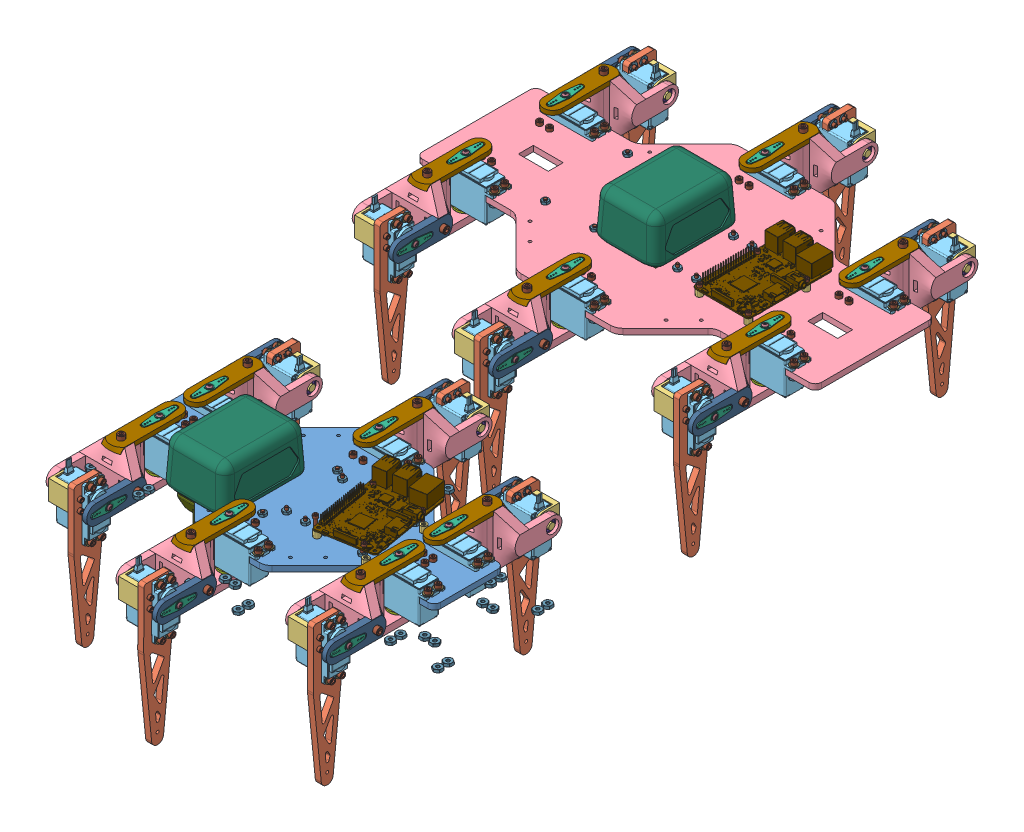
SolidWorks assembly Assem1, configuration Default. Lengths in mm.
Overall size (454.69 181.88 781.08).
774 component instances, 22 part files, 6 mates.
Components (placement in the parent):
- Hexapod_NewBody-1: Hexapod_NewBody [Défaut] at origin size (371.2 181.88 349.28)
  - Body_V2-5: Body_V2 [Default] at (-310 -5.6 15) x (1 0 0) z (0 1 0) size (310 170 5.6)
  - Leg-6: Leg [Default] at (-54.94 -26.67 -0.094) size (70.67 158.62 124.58)
    - Foot_V2_Straight-1: Foot_V2_Straight [Default] at (5.4563 4.661 -91.3712) x (0.005731 -0.001458 0.999983) z (-0.999984 0 0.005731) size (28 145.4 6)
    - bearing_mount_foot-1: bearing_mount_foot [Default] at (5.5782 16.6093 -99.7646) x (-0.005731 0.001458 -0.999983) z (0.999984 0 -0.005731) size (25 20 29.5)
    - Joint-1: Joint [Défaut] at (36.1468 26.4662 -54.5086) x (-0.005731 0 -0.999984) z (0 1 0) size (96.52 53.26 53.26)
    - hs-422-2: hs-422 [Défaut] at (5.505 6.6398 -77.4623) x (-0.005731 0.001458 -0.999983) z (0.000008 0.999999 0.001458) size (19.81 42.09 58.23)
    - hs-422-3: hs-422 [Défaut] at (19.939 20.701 -19.812) x (0 0 1) z (-1 0 0) size (19.81 42.09 58.23)
    - hs-422_horn_straight-1: hs-422_horn_straight [Default] at (-16.4246 16.9412 -87.2278) x (0.005731 0 0.999984) z (0 1 0) size (33.93 4.93 8.79)
    - hs-422_horn_straight-2: hs-422_horn_straight [Default] at (9.652 42.5743 -9.906) x (-0.005731 0 -0.999984) z (-0.999984 0 0.005731) size (33.93 4.93 8.79)
    - Bearing_mount_leg-1: Bearing_mount_leg [Default] at (9.652 21 2.594) x (0 0 1) z (0 -1 0) size (35 20 30)
    - Bearing-1: Bearing [Default] at (9.652 -6.7498 -9.906) x (0.84763 0 0.530588) z (-0.530588 0 0.84763) size (13.87 4.75 13.87)
    - Bearing-2: Bearing [Default] at (32.8986 16.9412 -87.5105) x (0.003061 -0.845349 0.534206) z (-0.004844 -0.534214 -0.845335) size (13.87 4.75 13.87)
    - Joint_attachment_leg-1: Joint_attachment_leg [Défaut] at (36.1468 26.4662 -54.5086) x (-0.005731 0 -0.999984) z (0 1 0) size (74.32 19.07 4.32)
    - Joint_attachment_foot-1: Joint_attachment_foot [Défaut] at (36.1468 26.4662 -54.5086) x (-0.005731 0 -0.999984) z (0 1 0) size (64.08 6.7 19.07)
    - socket_1_2_6-32_with_washer-1: socket_1_2_6-32_with_washer [Défaut] at (43.8172 -14.6702 -93.6435) x (0.999984 0 -0.005731) z (0.004959 -0.501262 0.865281) size (16.21 7.92 7.92)
      - socket head cap screw_ai-1: socket head cap screw_ai [HX-SHCS 0.138-32x0.5x0.5-N] at (-51.206 -1.62 2.0257) size (16.21 5.74 5.74)
      - flat washer type b narrow_ai-1: flat washer type b narrow_ai [Narrow FW 0.138] at (-46.888 -1.62 2.0257) size (0.81 7.92 7.92)
    - socket_1_2_6-32_with_washer-2: socket_1_2_6-32_with_washer [Défaut] at (43.8716 -19.1255 -84.1659) x (0.999984 0 -0.005731) z (0.000008 0.999999 0.001458) size (16.21 7.92 7.92)
      - socket head cap screw_ai-1: socket head cap screw_ai [HX-SHCS 0.138-32x0.5x0.5-N] at (-51.206 -1.62 2.0257) size (16.21 5.74 5.74)
      - flat washer type b narrow_ai-1: flat washer type b narrow_ai [Narrow FW 0.138] at (-46.888 -1.62 2.0257) size (0.81 7.92 7.92)
    - socket_1_2_6-32_with_washer-3: socket_1_2_6-32_with_washer [Défaut] at (43.8284 27.9935 -91.6928) x (0.999984 0 -0.005731) z (-0.004959 0.501262 -0.865281) size (16.21 7.92 7.92)
      - socket head cap screw_ai-1: socket head cap screw_ai [HX-SHCS 0.138-32x0.5x0.5-N] at (-51.206 -1.62 2.0257) size (16.21 5.74 5.74)
      - flat washer type b narrow_ai-1: flat washer type b narrow_ai [Narrow FW 0.138] at (-46.888 -1.62 2.0257) size (0.81 7.92 7.92)
    - socket_1_2_6-32_with_washer-4: socket_1_2_6-32_with_washer [Défaut] at (43.8866 27.9806 -81.533) x (0.999984 0 -0.005731) z (-0.004959 0.501262 -0.865281) size (16.21 7.92 7.92)
      - socket head cap screw_ai-1: socket head cap screw_ai [HX-SHCS 0.138-32x0.5x0.5-N] at (-51.206 -1.62 2.0257) size (16.21 5.74 5.74)
      - flat washer type b narrow_ai-1: flat washer type b narrow_ai [Narrow FW 0.138] at (-46.888 -1.62 2.0257) size (0.81 7.92 7.92)
    - socket button head cap screw_ai-2: socket button head cap screw_ai [SBHCSCREW 0.112-40x0.25-HX-N] at (-19.4218 16.9412 -87.2107) x (0.999984 0 -0.005731) z (-0.002865 0.866025 -0.499992) size (7.85 5.41 5.41)
    - socket button head cap screw_ai-3: socket button head cap screw_ai [SBHCSCREW 0.112-40x0.25-HX-N] at (9.652 45.5715 -9.906) x (0 -1 0) z (0.868877 0 0.495029) size (7.85 5.41 5.41)
    - machine screw nut hex_ai-7: machine screw nut hex_ai [MSHXNUT 0.138-32-D-N] at (5.4499 -17.0874 -92.4829) x (-0.004959 0.501262 -0.865281) z (0.999984 0 -0.005731) size (7.92 9.15 2.9)
    - machine screw nut hex_ai-8: machine screw nut hex_ai [MSHXNUT 0.138-32-D-N] at (5.5081 -17.1022 -82.3231) x (-0.004959 0.501262 -0.865281) z (-0.999984 0 0.005731) size (7.92 9.15 2.9)
    - machine screw nut hex_ai-9: machine screw nut hex_ai [MSHXNUT 0.138-32-D-N] at (5.4503 30.4106 -92.4136) x (0.000008 0.999999 0.001458) z (0.999984 0 -0.005731) size (7.92 9.15 2.9)
    - machine screw nut hex_ai-10: machine screw nut hex_ai [MSHXNUT 0.138-32-D-N] at (5.5085 30.3978 -82.2538) x (0.000008 0.999999 0.001458) z (0.999984 0 -0.005731) size (7.92 9.15 2.9)
    - socket head cap screw_ai-1: socket head cap screw_ai [HX-SHCS 0.164-32x0.5x0.5-N] at (9.4314 47.8568 -48.4033) x (0 -1 0) z (0.005731 0 0.999984) size (16.87 6.86 6.86)
    - socket head cap screw_ai-2: socket head cap screw_ai [HX-SHCS 0.164-32x0.5x0.5-N] at (-21.5482 16.9412 -59.4711) x (0.999984 0 -0.005731) z (0.005731 0 0.999984) size (16.87 6.86 6.86)
    - machine screw nut hex_ai-11: machine screw nut hex_ai [MSHXNUT 0.164-32-D-N] at (9.4314 33.127 -48.4033) x (0.868877 0 0.495029) z (0 1 0) size (8.74 10.09 3.3)
    - machine screw nut hex_ai-12: machine screw nut hex_ai [MSHXNUT 0.164-32-D-N] at (-6.8186 16.9412 -59.5556) x (0.005731 0 0.999984) z (-0.999984 0 0.005731) size (8.74 10.09 3.3)
    - socket head cap screw_ai-3: socket head cap screw_ai [HX-SHCS 0.112-40x0.5x0.5-N] at (-3.4365 11.6733 -99.7202) x (0.999984 0 -0.005731) z (0.005731 -0.001458 0.999983) size (15.54 4.65 4.65)
    - socket head cap screw_ai-4: socket head cap screw_ai [HX-SHCS 0.112-40x0.5x0.5-N] at (-3.4364 21.6733 -99.7056) x (0.999984 0 -0.005731) z (-0.005731 0.001458 -0.999983) size (15.54 4.65 4.65)
    - socket_1_2_6-32_with_washer-5: socket_1_2_6-32_with_washer [Défaut] at (-3.4199 -17.7034 -7.3903) x (0 -1 0) z (0.5 0 0.866025) size (16.21 7.92 7.92)
      - socket head cap screw_ai-1: socket head cap screw_ai [HX-SHCS 0.138-32x0.5x0.5-N] at (-51.206 -1.62 2.0257) size (16.21 5.74 5.74)
      - flat washer type b narrow_ai-1: flat washer type b narrow_ai [Narrow FW 0.138] at (-46.888 -1.62 2.0257) size (0.81 7.92 7.92)
    - socket_1_2_6-32_with_washer-6: socket_1_2_6-32_with_washer [Défaut] at (44.0781 -17.7034 -17.5503) x (0 -1 0) z (0.5 0 0.866025) size (16.21 7.92 7.92)
      - socket head cap screw_ai-1: socket head cap screw_ai [HX-SHCS 0.138-32x0.5x0.5-N] at (-51.206 -1.62 2.0257) size (16.21 5.74 5.74)
      - flat washer type b narrow_ai-1: flat washer type b narrow_ai [Narrow FW 0.138] at (-46.888 -1.62 2.0257) size (0.81 7.92 7.92)
    - socket_1_2_6-32_with_washer-7: socket_1_2_6-32_with_washer [Défaut] at (-3.4199 -17.7034 -17.5503) x (0 -1 0) z (0.5 0 0.866025) size (16.21 7.92 7.92)
      - socket head cap screw_ai-1: socket head cap screw_ai [HX-SHCS 0.138-32x0.5x0.5-N] at (-51.206 -1.62 2.0257) size (16.21 5.74 5.74)
      - flat washer type b narrow_ai-1: flat washer type b narrow_ai [Narrow FW 0.138] at (-46.888 -1.62 2.0257) size (0.81 7.92 7.92)
    - socket_1_2_6-32_with_washer-8: socket_1_2_6-32_with_washer [Défaut] at (44.0781 -17.7034 -7.3903) x (0 -1 0) z (0.5 0 0.866025) size (16.21 7.92 7.92)
      - socket head cap screw_ai-1: socket head cap screw_ai [HX-SHCS 0.138-32x0.5x0.5-N] at (-51.206 -1.62 2.0257) size (16.21 5.74 5.74)
      - flat washer type b narrow_ai-1: flat washer type b narrow_ai [Narrow FW 0.138] at (-46.888 -1.62 2.0257) size (0.81 7.92 7.92)
  - Leg-7: Leg [Default] at (-294.94 -26.67 -0.094) size (70.67 158.62 124.58)
    - Foot_V2_Straight-1: Foot_V2_Straight [Default] at (5.4563 4.661 -91.3712) x (0.005731 -0.001458 0.999983) z (-0.999984 0 0.005731) size (28 145.4 6)
    - bearing_mount_foot-1: bearing_mount_foot [Default] at (5.5782 16.6093 -99.7646) x (-0.005731 0.001458 -0.999983) z (0.999984 0 -0.005731) size (25 20 29.5)
    - Joint-1: Joint [Défaut] at (36.1468 26.4662 -54.5086) x (-0.005731 0 -0.999984) z (0 1 0) size (96.52 53.26 53.26)
    - hs-422-2: hs-422 [Défaut] at (5.505 6.6398 -77.4623) x (-0.005731 0.001458 -0.999983) z (0.000008 0.999999 0.001458) size (19.81 42.09 58.23)
    - hs-422-3: hs-422 [Défaut] at (19.939 20.701 -19.812) x (0 0 1) z (-1 0 0) size (19.81 42.09 58.23)
    - hs-422_horn_straight-1: hs-422_horn_straight [Default] at (-16.4246 16.9412 -87.2278) x (0.005731 0 0.999984) z (0 1 0) size (33.93 4.93 8.79)
    - hs-422_horn_straight-2: hs-422_horn_straight [Default] at (9.652 42.5743 -9.906) x (-0.005731 0 -0.999984) z (-0.999984 0 0.005731) size (33.93 4.93 8.79)
    - Bearing_mount_leg-1: Bearing_mount_leg [Default] at (9.652 21 2.594) x (0 0 1) z (0 -1 0) size (35 20 30)
    - Bearing-1: Bearing [Default] at (9.652 -6.7498 -9.906) x (0.84763 0 0.530588) z (-0.530588 0 0.84763) size (13.87 4.75 13.87)
    - Bearing-2: Bearing [Default] at (32.8986 16.9412 -87.5105) x (0.003061 -0.845349 0.534206) z (-0.004844 -0.534214 -0.845335) size (13.87 4.75 13.87)
    - Joint_attachment_leg-1: Joint_attachment_leg [Défaut] at (36.1468 26.4662 -54.5086) x (-0.005731 0 -0.999984) z (0 1 0) size (74.32 19.07 4.32)
    - Joint_attachment_foot-1: Joint_attachment_foot [Défaut] at (36.1468 26.4662 -54.5086) x (-0.005731 0 -0.999984) z (0 1 0) size (64.08 6.7 19.07)
    - socket_1_2_6-32_with_washer-1: socket_1_2_6-32_with_washer [Défaut] at (43.8172 -14.6702 -93.6435) x (0.999984 0 -0.005731) z (0.004959 -0.501262 0.865281) size (16.21 7.92 7.92)
      - socket head cap screw_ai-1: socket head cap screw_ai [HX-SHCS 0.138-32x0.5x0.5-N] at (-51.206 -1.62 2.0257) size (16.21 5.74 5.74)
      - flat washer type b narrow_ai-1: flat washer type b narrow_ai [Narrow FW 0.138] at (-46.888 -1.62 2.0257) size (0.81 7.92 7.92)
    - socket_1_2_6-32_with_washer-2: socket_1_2_6-32_with_washer [Défaut] at (43.8716 -19.1255 -84.1659) x (0.999984 0 -0.005731) z (0.000008 0.999999 0.001458) size (16.21 7.92 7.92)
      - socket head cap screw_ai-1: socket head cap screw_ai [HX-SHCS 0.138-32x0.5x0.5-N] at (-51.206 -1.62 2.0257) size (16.21 5.74 5.74)
      - flat washer type b narrow_ai-1: flat washer type b narrow_ai [Narrow FW 0.138] at (-46.888 -1.62 2.0257) size (0.81 7.92 7.92)
    - socket_1_2_6-32_with_washer-3: socket_1_2_6-32_with_washer [Défaut] at (43.8284 27.9935 -91.6928) x (0.999984 0 -0.005731) z (-0.004959 0.501262 -0.865281) size (16.21 7.92 7.92)
      - socket head cap screw_ai-1: socket head cap screw_ai [HX-SHCS 0.138-32x0.5x0.5-N] at (-51.206 -1.62 2.0257) size (16.21 5.74 5.74)
      - flat washer type b narrow_ai-1: flat washer type b narrow_ai [Narrow FW 0.138] at (-46.888 -1.62 2.0257) size (0.81 7.92 7.92)
    - socket_1_2_6-32_with_washer-4: socket_1_2_6-32_with_washer [Défaut] at (43.8866 27.9806 -81.533) x (0.999984 0 -0.005731) z (-0.004959 0.501262 -0.865281) size (16.21 7.92 7.92)
      - socket head cap screw_ai-1: socket head cap screw_ai [HX-SHCS 0.138-32x0.5x0.5-N] at (-51.206 -1.62 2.0257) size (16.21 5.74 5.74)
      - flat washer type b narrow_ai-1: flat washer type b narrow_ai [Narrow FW 0.138] at (-46.888 -1.62 2.0257) size (0.81 7.92 7.92)
    - socket button head cap screw_ai-2: socket button head cap screw_ai [SBHCSCREW 0.112-40x0.25-HX-N] at (-19.4218 16.9412 -87.2107) x (0.999984 0 -0.005731) z (-0.002865 0.866025 -0.499992) size (7.85 5.41 5.41)
    - socket button head cap screw_ai-3: socket button head cap screw_ai [SBHCSCREW 0.112-40x0.25-HX-N] at (9.652 45.5715 -9.906) x (0 -1 0) z (0.868877 0 0.495029) size (7.85 5.41 5.41)
    - machine screw nut hex_ai-7: machine screw nut hex_ai [MSHXNUT 0.138-32-D-N] at (5.4499 -17.0874 -92.4829) x (-0.004959 0.501262 -0.865281) z (0.999984 0 -0.005731) size (7.92 9.15 2.9)
    - machine screw nut hex_ai-8: machine screw nut hex_ai [MSHXNUT 0.138-32-D-N] at (5.5081 -17.1022 -82.3231) x (-0.004959 0.501262 -0.865281) z (-0.999984 0 0.005731) size (7.92 9.15 2.9)
    - machine screw nut hex_ai-9: machine screw nut hex_ai [MSHXNUT 0.138-32-D-N] at (5.4503 30.4106 -92.4136) x (0.000008 0.999999 0.001458) z (0.999984 0 -0.005731) size (7.92 9.15 2.9)
    - machine screw nut hex_ai-10: machine screw nut hex_ai [MSHXNUT 0.138-32-D-N] at (5.5085 30.3978 -82.2538) x (0.000008 0.999999 0.001458) z (0.999984 0 -0.005731) size (7.92 9.15 2.9)
    - socket head cap screw_ai-1: socket head cap screw_ai [HX-SHCS 0.164-32x0.5x0.5-N] at (9.4314 47.8568 -48.4033) x (0 -1 0) z (0.005731 0 0.999984) size (16.87 6.86 6.86)
    - socket head cap screw_ai-2: socket head cap screw_ai [HX-SHCS 0.164-32x0.5x0.5-N] at (-21.5482 16.9412 -59.4711) x (0.999984 0 -0.005731) z (0.005731 0 0.999984) size (16.87 6.86 6.86)
    - machine screw nut hex_ai-11: machine screw nut hex_ai [MSHXNUT 0.164-32-D-N] at (9.4314 33.127 -48.4033) x (0.868877 0 0.495029) z (0 1 0) size (8.74 10.09 3.3)
    - machine screw nut hex_ai-12: machine screw nut hex_ai [MSHXNUT 0.164-32-D-N] at (-6.8186 16.9412 -59.5556) x (0.005731 0 0.999984) z (-0.999984 0 0.005731) size (8.74 10.09 3.3)
    - socket head cap screw_ai-3: socket head cap screw_ai [HX-SHCS 0.112-40x0.5x0.5-N] at (-3.4365 11.6733 -99.7202) x (0.999984 0 -0.005731) z (0.005731 -0.001458 0.999983) size (15.54 4.65 4.65)
    - socket head cap screw_ai-4: socket head cap screw_ai [HX-SHCS 0.112-40x0.5x0.5-N] at (-3.4364 21.6733 -99.7056) x (0.999984 0 -0.005731) z (-0.005731 0.001458 -0.999983) size (15.54 4.65 4.65)
    - socket_1_2_6-32_with_washer-5: socket_1_2_6-32_with_washer [Défaut] at (-3.4199 -17.7034 -7.3903) x (0 -1 0) z (0.5 0 0.866025) size (16.21 7.92 7.92)
      - socket head cap screw_ai-1: socket head cap screw_ai [HX-SHCS 0.138-32x0.5x0.5-N] at (-51.206 -1.62 2.0257) size (16.21 5.74 5.74)
      - flat washer type b narrow_ai-1: flat washer type b narrow_ai [Narrow FW 0.138] at (-46.888 -1.62 2.0257) size (0.81 7.92 7.92)
    - socket_1_2_6-32_with_washer-6: socket_1_2_6-32_with_washer [Défaut] at (44.0781 -17.7034 -17.5503) x (0 -1 0) z (0.5 0 0.866025) size (16.21 7.92 7.92)
      - socket head cap screw_ai-1: socket head cap screw_ai [HX-SHCS 0.138-32x0.5x0.5-N] at (-51.206 -1.62 2.0257) size (16.21 5.74 5.74)
      - flat washer type b narrow_ai-1: flat washer type b narrow_ai [Narrow FW 0.138] at (-46.888 -1.62 2.0257) size (0.81 7.92 7.92)
    - socket_1_2_6-32_with_washer-7: socket_1_2_6-32_with_washer [Défaut] at (-3.4199 -17.7034 -17.5503) x (0 -1 0) z (0.5 0 0.866025) size (16.21 7.92 7.92)
      - socket head cap screw_ai-1: socket head cap screw_ai [HX-SHCS 0.138-32x0.5x0.5-N] at (-51.206 -1.62 2.0257) size (16.21 5.74 5.74)
      - flat washer type b narrow_ai-1: flat washer type b narrow_ai [Narrow FW 0.138] at (-46.888 -1.62 2.0257) size (0.81 7.92 7.92)
    - socket_1_2_6-32_with_washer-8: socket_1_2_6-32_with_washer [Défaut] at (44.0781 -17.7034 -7.3903) x (0 -1 0) z (0.5 0 0.866025) size (16.21 7.92 7.92)
      - socket head cap screw_ai-1: socket head cap screw_ai [HX-SHCS 0.138-32x0.5x0.5-N] at (-51.206 -1.62 2.0257) size (16.21 5.74 5.74)
      - flat washer type b narrow_ai-1: flat washer type b narrow_ai [Narrow FW 0.138] at (-46.888 -1.62 2.0257) size (0.81 7.92 7.92)
  - Leg-8: Leg [Default] at (-174.94 -26.67 -50.094) size (70.67 158.62 124.58)
    - Foot_V2_Straight-1: Foot_V2_Straight [Default] at (5.4563 4.661 -91.3712) x (0.005731 -0.001458 0.999983) z (-0.999984 0 0.005731) size (28 145.4 6)
    - bearing_mount_foot-1: bearing_mount_foot [Default] at (5.5782 16.6093 -99.7646) x (-0.005731 0.001458 -0.999983) z (0.999984 0 -0.005731) size (25 20 29.5)
    - Joint-1: Joint [Défaut] at (36.1468 26.4662 -54.5086) x (-0.005731 0 -0.999984) z (0 1 0) size (96.52 53.26 53.26)
    - hs-422-2: hs-422 [Défaut] at (5.505 6.6398 -77.4623) x (-0.005731 0.001458 -0.999983) z (0.000008 0.999999 0.001458) size (19.81 42.09 58.23)
    - hs-422-3: hs-422 [Défaut] at (19.939 20.701 -19.812) x (0 0 1) z (-1 0 0) size (19.81 42.09 58.23)
    - hs-422_horn_straight-1: hs-422_horn_straight [Default] at (-16.4246 16.9412 -87.2278) x (0.005731 0 0.999984) z (0 1 0) size (33.93 4.93 8.79)
    - hs-422_horn_straight-2: hs-422_horn_straight [Default] at (9.652 42.5743 -9.906) x (-0.005731 0 -0.999984) z (-0.999984 0 0.005731) size (33.93 4.93 8.79)
    - Bearing_mount_leg-1: Bearing_mount_leg [Default] at (9.652 21 2.594) x (0 0 1) z (0 -1 0) size (35 20 30)
    - Bearing-1: Bearing [Default] at (9.652 -6.7498 -9.906) x (0.84763 0 0.530588) z (-0.530588 0 0.84763) size (13.87 4.75 13.87)
    - Bearing-2: Bearing [Default] at (32.8986 16.9412 -87.5105) x (0.003061 -0.845349 0.534206) z (-0.004844 -0.534214 -0.845335) size (13.87 4.75 13.87)
    - Joint_attachment_leg-1: Joint_attachment_leg [Défaut] at (36.1468 26.4662 -54.5086) x (-0.005731 0 -0.999984) z (0 1 0) size (74.32 19.07 4.32)
    - Joint_attachment_foot-1: Joint_attachment_foot [Défaut] at (36.1468 26.4662 -54.5086) x (-0.005731 0 -0.999984) z (0 1 0) size (64.08 6.7 19.07)
    - socket_1_2_6-32_with_washer-1: socket_1_2_6-32_with_washer [Défaut] at (43.8172 -14.6702 -93.6435) x (0.999984 0 -0.005731) z (0.004959 -0.501262 0.865281) size (16.21 7.92 7.92)
      - socket head cap screw_ai-1: socket head cap screw_ai [HX-SHCS 0.138-32x0.5x0.5-N] at (-51.206 -1.62 2.0257) size (16.21 5.74 5.74)
      - flat washer type b narrow_ai-1: flat washer type b narrow_ai [Narrow FW 0.138] at (-46.888 -1.62 2.0257) size (0.81 7.92 7.92)
    - socket_1_2_6-32_with_washer-2: socket_1_2_6-32_with_washer [Défaut] at (43.8716 -19.1255 -84.1659) x (0.999984 0 -0.005731) z (0.000008 0.999999 0.001458) size (16.21 7.92 7.92)
      - socket head cap screw_ai-1: socket head cap screw_ai [HX-SHCS 0.138-32x0.5x0.5-N] at (-51.206 -1.62 2.0257) size (16.21 5.74 5.74)
      - flat washer type b narrow_ai-1: flat washer type b narrow_ai [Narrow FW 0.138] at (-46.888 -1.62 2.0257) size (0.81 7.92 7.92)
    - socket_1_2_6-32_with_washer-3: socket_1_2_6-32_with_washer [Défaut] at (43.8284 27.9935 -91.6928) x (0.999984 0 -0.005731) z (-0.004959 0.501262 -0.865281) size (16.21 7.92 7.92)
      - socket head cap screw_ai-1: socket head cap screw_ai [HX-SHCS 0.138-32x0.5x0.5-N] at (-51.206 -1.62 2.0257) size (16.21 5.74 5.74)
      - flat washer type b narrow_ai-1: flat washer type b narrow_ai [Narrow FW 0.138] at (-46.888 -1.62 2.0257) size (0.81 7.92 7.92)
    - socket_1_2_6-32_with_washer-4: socket_1_2_6-32_with_washer [Défaut] at (43.8866 27.9806 -81.533) x (0.999984 0 -0.005731) z (-0.004959 0.501262 -0.865281) size (16.21 7.92 7.92)
      - socket head cap screw_ai-1: socket head cap screw_ai [HX-SHCS 0.138-32x0.5x0.5-N] at (-51.206 -1.62 2.0257) size (16.21 5.74 5.74)
      - flat washer type b narrow_ai-1: flat washer type b narrow_ai [Narrow FW 0.138] at (-46.888 -1.62 2.0257) size (0.81 7.92 7.92)
    - socket button head cap screw_ai-2: socket button head cap screw_ai [SBHCSCREW 0.112-40x0.25-HX-N] at (-19.4218 16.9412 -87.2107) x (0.999984 0 -0.005731) z (-0.002865 0.866025 -0.499992) size (7.85 5.41 5.41)
    - socket button head cap screw_ai-3: socket button head cap screw_ai [SBHCSCREW 0.112-40x0.25-HX-N] at (9.652 45.5715 -9.906) x (0 -1 0) z (0.868877 0 0.495029) size (7.85 5.41 5.41)
    - machine screw nut hex_ai-7: machine screw nut hex_ai [MSHXNUT 0.138-32-D-N] at (5.4499 -17.0874 -92.4829) x (-0.004959 0.501262 -0.865281) z (0.999984 0 -0.005731) size (7.92 9.15 2.9)
    - machine screw nut hex_ai-8: machine screw nut hex_ai [MSHXNUT 0.138-32-D-N] at (5.5081 -17.1022 -82.3231) x (-0.004959 0.501262 -0.865281) z (-0.999984 0 0.005731) size (7.92 9.15 2.9)
    - machine screw nut hex_ai-9: machine screw nut hex_ai [MSHXNUT 0.138-32-D-N] at (5.4503 30.4106 -92.4136) x (0.000008 0.999999 0.001458) z (0.999984 0 -0.005731) size (7.92 9.15 2.9)
    - machine screw nut hex_ai-10: machine screw nut hex_ai [MSHXNUT 0.138-32-D-N] at (5.5085 30.3978 -82.2538) x (0.000008 0.999999 0.001458) z (0.999984 0 -0.005731) size (7.92 9.15 2.9)
    - socket head cap screw_ai-1: socket head cap screw_ai [HX-SHCS 0.164-32x0.5x0.5-N] at (9.4314 47.8568 -48.4033) x (0 -1 0) z (0.005731 0 0.999984) size (16.87 6.86 6.86)
    - socket head cap screw_ai-2: socket head cap screw_ai [HX-SHCS 0.164-32x0.5x0.5-N] at (-21.5482 16.9412 -59.4711) x (0.999984 0 -0.005731) z (0.005731 0 0.999984) size (16.87 6.86 6.86)
    - machine screw nut hex_ai-11: machine screw nut hex_ai [MSHXNUT 0.164-32-D-N] at (9.4314 33.127 -48.4033) x (0.868877 0 0.495029) z (0 1 0) size (8.74 10.09 3.3)
    - machine screw nut hex_ai-12: machine screw nut hex_ai [MSHXNUT 0.164-32-D-N] at (-6.8186 16.9412 -59.5556) x (0.005731 0 0.999984) z (-0.999984 0 0.005731) size (8.74 10.09 3.3)
    - socket head cap screw_ai-3: socket head cap screw_ai [HX-SHCS 0.112-40x0.5x0.5-N] at (-3.4365 11.6733 -99.7202) x (0.999984 0 -0.005731) z (0.005731 -0.001458 0.999983) size (15.54 4.65 4.65)
    - socket head cap screw_ai-4: socket head cap screw_ai [HX-SHCS 0.112-40x0.5x0.5-N] at (-3.4364 21.6733 -99.7056) x (0.999984 0 -0.005731) z (-0.005731 0.001458 -0.999983) size (15.54 4.65 4.65)
    - socket_1_2_6-32_with_washer-5: socket_1_2_6-32_with_washer [Défaut] at (-3.4199 -17.7034 -7.3903) x (0 -1 0) z (0.5 0 0.866025) size (16.21 7.92 7.92)
      - socket head cap screw_ai-1: socket head cap screw_ai [HX-SHCS 0.138-32x0.5x0.5-N] at (-51.206 -1.62 2.0257) size (16.21 5.74 5.74)
      - flat washer type b narrow_ai-1: flat washer type b narrow_ai [Narrow FW 0.138] at (-46.888 -1.62 2.0257) size (0.81 7.92 7.92)
    - socket_1_2_6-32_with_washer-6: socket_1_2_6-32_with_washer [Défaut] at (44.0781 -17.7034 -17.5503) x (0 -1 0) z (0.5 0 0.866025) size (16.21 7.92 7.92)
      - socket head cap screw_ai-1: socket head cap screw_ai [HX-SHCS 0.138-32x0.5x0.5-N] at (-51.206 -1.62 2.0257) size (16.21 5.74 5.74)
      - flat washer type b narrow_ai-1: flat washer type b narrow_ai [Narrow FW 0.138] at (-46.888 -1.62 2.0257) size (0.81 7.92 7.92)
    - socket_1_2_6-32_with_washer-7: socket_1_2_6-32_with_washer [Défaut] at (-3.4199 -17.7034 -17.5503) x (0 -1 0) z (0.5 0 0.866025) size (16.21 7.92 7.92)
      - socket head cap screw_ai-1: socket head cap screw_ai [HX-SHCS 0.138-32x0.5x0.5-N] at (-51.206 -1.62 2.0257) size (16.21 5.74 5.74)
      - flat washer type b narrow_ai-1: flat washer type b narrow_ai [Narrow FW 0.138] at (-46.888 -1.62 2.0257) size (0.81 7.92 7.92)
    - socket_1_2_6-32_with_washer-8: socket_1_2_6-32_with_washer [Défaut] at (44.0781 -17.7034 -7.3903) x (0 -1 0) z (0.5 0 0.866025) size (16.21 7.92 7.92)
      - socket head cap screw_ai-1: socket head cap screw_ai [HX-SHCS 0.138-32x0.5x0.5-N] at (-51.206 -1.62 2.0257) size (16.21 5.74 5.74)
      - flat washer type b narrow_ai-1: flat washer type b narrow_ai [Narrow FW 0.138] at (-46.888 -1.62 2.0257) size (0.81 7.92 7.92)
  - Leg_V2(Mirror)-4: Leg_V2(Mirror) [Default] at (-294.94 -26.67 30.094) x (-1 0 0) z (0 0 -1) size (66.23 158.62 124.7)
    - Foot_V2_Straight-1: Foot_V2_Straight [Default] at (-13.3652 4.661 -91.3946) x (-0.000191 -0.001458 0.999999) z (-1 0 -0.000191) size (28 145.4 6)
    - bearing_mount_foot-1: bearing_mount_foot [Default] at (-13.1936 16.6093 -99.7872) x (0.000191 0.001458 -0.999999) z (1 0 0.000191) size (25 20 29.5)
    - Joint-1: Joint [Défaut] at (17.1065 26.4662 -54.3509) x (0.000191 0 -1) z (0 1 0) size (96.52 53.26 53.26)
    - hs-422-2: hs-422 [Défaut] at (-13.3989 6.6398 -77.4857) x (0.000191 0.001458 -0.999999) z (0 0.999999 0.001458) size (19.81 42.09 58.23)
    - hs-422-3: hs-422 [Défaut] at (-19.939 20.701 0) x (0 0 -1) z (1 0 0) size (19.81 42.09 58.23)
    - hs-422_horn_straight-1: hs-422_horn_straight [Default] at (-35.2703 16.9412 -87.3809) x (-0.000191 0 1) z (0 1 0) size (33.93 4.93 8.79)
    - hs-422_horn_straight-2: hs-422_horn_straight [Default] at (-9.652 42.5743 -9.906) x (0.000191 0 -1) z (-1 0 -0.000191) size (33.93 4.93 8.79)
    - Bearing_mount_leg-1: Bearing_mount_leg [Default] at (-9.652 21 2.594) x (0 0 1) z (0 -1 0) size (35 20 30)
    - Bearing-1: Bearing [Default] at (-9.652 -6.7498 -9.906) x (0.84763 0 0.530588) z (-0.530588 0 0.84763) size (13.87 4.75 13.87)
    - Bearing-2: Bearing [Default] at (14.0538 16.9412 -87.3715) x (-0.000107 0.826531 0.562891) z (-0.000158 -0.562891 0.826531) size (13.87 4.75 13.87)
    - Joint_attachment_leg-1: Joint_attachment_leg [Défaut] at (17.1065 26.4662 -54.3509) x (0.000191 0 -1) z (0 1 0) size (74.32 19.07 4.32)
    - Joint_attachment_foot-1: Joint_attachment_foot [Défaut] at (17.1065 26.4662 -54.3509) x (0.000191 0 -1) z (0 1 0) size (64.08 6.7 19.07)
    - socket_1_2_6-32_with_washer-1: socket_1_2_6-32_with_washer [Défaut] at (25.0085 -14.6702 -93.4398) x (1 0 0.000191) z (-0.000165 -0.501262 0.865296) size (16.21 7.92 7.92)
      - socket head cap screw_ai-1: socket head cap screw_ai [HX-SHCS 0.138-32x0.5x0.5-N] at (-51.206 -1.62 2.0257) size (16.21 5.74 5.74)
      - flat washer type b narrow_ai-1: flat washer type b narrow_ai [Narrow FW 0.138] at (-46.888 -1.62 2.0257) size (0.81 7.92 7.92)
    - socket_1_2_6-32_with_washer-2: socket_1_2_6-32_with_washer [Défaut] at (25.0067 -19.1255 -83.9619) x (1 0 0.000191) z (0 0.999999 0.001458) size (16.21 7.92 7.92)
      - socket head cap screw_ai-1: socket head cap screw_ai [HX-SHCS 0.138-32x0.5x0.5-N] at (-51.206 -1.62 2.0257) size (16.21 5.74 5.74)
      - flat washer type b narrow_ai-1: flat washer type b narrow_ai [Narrow FW 0.138] at (-46.888 -1.62 2.0257) size (0.81 7.92 7.92)
    - socket_1_2_6-32_with_washer-3: socket_1_2_6-32_with_washer [Défaut] at (25.0081 27.9935 -91.489) x (1 0 0.000191) z (0.000165 0.501262 -0.865296) size (16.21 7.92 7.92)
      - socket head cap screw_ai-1: socket head cap screw_ai [HX-SHCS 0.138-32x0.5x0.5-N] at (-51.206 -1.62 2.0257) size (16.21 5.74 5.74)
      - flat washer type b narrow_ai-1: flat washer type b narrow_ai [Narrow FW 0.138] at (-46.888 -1.62 2.0257) size (0.81 7.92 7.92)
    - socket_1_2_6-32_with_washer-4: socket_1_2_6-32_with_washer [Défaut] at (25.0062 27.9806 -81.329) x (1 0 0.000191) z (0.000165 0.501262 -0.865296) size (16.21 7.92 7.92)
      - socket head cap screw_ai-1: socket head cap screw_ai [HX-SHCS 0.138-32x0.5x0.5-N] at (-51.206 -1.62 2.0257) size (16.21 5.74 5.74)
      - flat washer type b narrow_ai-1: flat washer type b narrow_ai [Narrow FW 0.138] at (-46.888 -1.62 2.0257) size (0.81 7.92 7.92)
    - socket button head cap screw_ai-2: socket button head cap screw_ai [SBHCSCREW 0.112-40x0.25-HX-N] at (-38.2675 16.9412 -87.3815) x (1 0 0.000191) z (0.000095 0.866025 -0.5) size (7.85 5.41 5.41)
    - socket button head cap screw_ai-3: socket button head cap screw_ai [SBHCSCREW 0.112-40x0.25-HX-N] at (-9.652 45.5715 -9.906) x (0 -1 0) z (0.86593 0 0.500165) size (7.85 5.41 5.41)
    - machine screw nut hex_ai-7: machine screw nut hex_ai [MSHXNUT 0.138-32-D-N] at (-13.365 -17.0874 -92.5063) x (0.000165 0.501262 -0.865296) z (1 0 0.000191) size (7.92 9.15 2.9)
    - machine screw nut hex_ai-8: machine screw nut hex_ai [MSHXNUT 0.138-32-D-N] at (-13.367 -17.1022 -82.3463) x (0.000165 0.501262 -0.865296) z (-1 0 -0.000191) size (7.92 9.15 2.9)
    - machine screw nut hex_ai-9: machine screw nut hex_ai [MSHXNUT 0.138-32-D-N] at (-13.3651 30.4106 -92.4371) x (0 0.999999 0.001458) z (1 0 0.000191) size (7.92 9.15 2.9)
    - machine screw nut hex_ai-10: machine screw nut hex_ai [MSHXNUT 0.138-32-D-N] at (-13.367 30.3978 -82.2771) x (0 0.999999 0.001458) z (1 0 0.000191) size (7.92 9.15 2.9)
    - socket head cap screw_ai-1: socket head cap screw_ai [HX-SHCS 0.164-32x0.5x0.5-N] at (-9.6447 47.8568 -48.4039) x (0 -1 0) z (-0.000191 0 1) size (16.87 6.86 6.86)
    - socket head cap screw_ai-2: socket head cap screw_ai [HX-SHCS 0.164-32x0.5x0.5-N] at (-40.5581 16.9412 -59.655) x (1 0 0.000191) z (-0.000191 0 1) size (16.87 6.86 6.86)
    - machine screw nut hex_ai-11: machine screw nut hex_ai [MSHXNUT 0.164-32-D-N] at (-9.6447 33.127 -48.4039) x (0.86593 0 0.500165) z (0 1 0) size (8.74 10.09 3.3)
    - machine screw nut hex_ai-12: machine screw nut hex_ai [MSHXNUT 0.164-32-D-N] at (-25.8283 16.9412 -59.6522) x (-0.000191 0 1) z (-1 0 -0.000191) size (8.74 10.09 3.3)
    - socket head cap screw_ai-3: socket head cap screw_ai [HX-SHCS 0.112-40x0.5x0.5-N] at (-22.2084 11.6733 -99.7961) x (1 0 0.000191) z (-0.000191 -0.001458 0.999999) size (15.54 4.65 4.65)
    - socket head cap screw_ai-4: socket head cap screw_ai [HX-SHCS 0.112-40x0.5x0.5-N] at (-22.2084 21.6733 -99.7815) x (1 0 0.000191) z (0.000191 0.001458 -0.999999) size (15.54 4.65 4.65)
    - socket_1_2_6-32_with_washer-5: socket_1_2_6-32_with_washer [Défaut] at (3.4199 -17.7034 -12.4217) x (0 -1 0) z (-0.5 0 -0.866025) size (16.21 7.92 7.92)
      - socket head cap screw_ai-1: socket head cap screw_ai [HX-SHCS 0.138-32x0.5x0.5-N] at (-51.206 -1.62 2.0257) size (16.21 5.74 5.74)
      - flat washer type b narrow_ai-1: flat washer type b narrow_ai [Narrow FW 0.138] at (-46.888 -1.62 2.0257) size (0.81 7.92 7.92)
    - socket_1_2_6-32_with_washer-6: socket_1_2_6-32_with_washer [Défaut] at (-44.0781 -17.7034 -2.2617) x (0 -1 0) z (-0.5 0 -0.866025) size (16.21 7.92 7.92)
      - socket head cap screw_ai-1: socket head cap screw_ai [HX-SHCS 0.138-32x0.5x0.5-N] at (-51.206 -1.62 2.0257) size (16.21 5.74 5.74)
      - flat washer type b narrow_ai-1: flat washer type b narrow_ai [Narrow FW 0.138] at (-46.888 -1.62 2.0257) size (0.81 7.92 7.92)
    - socket_1_2_6-32_with_washer-7: socket_1_2_6-32_with_washer [Défaut] at (3.4199 -17.7034 -2.2617) x (0 -1 0) z (-0.5 0 -0.866025) size (16.21 7.92 7.92)
      - socket head cap screw_ai-1: socket head cap screw_ai [HX-SHCS 0.138-32x0.5x0.5-N] at (-51.206 -1.62 2.0257) size (16.21 5.74 5.74)
      - flat washer type b narrow_ai-1: flat washer type b narrow_ai [Narrow FW 0.138] at (-46.888 -1.62 2.0257) size (0.81 7.92 7.92)
    - socket_1_2_6-32_with_washer-8: socket_1_2_6-32_with_washer [Défaut] at (-44.0781 -17.7034 -12.4217) x (0 -1 0) z (-0.5 0 -0.866025) size (16.21 7.92 7.92)
      - socket head cap screw_ai-1: socket head cap screw_ai [HX-SHCS 0.138-32x0.5x0.5-N] at (-51.206 -1.62 2.0257) size (16.21 5.74 5.74)
      - flat washer type b narrow_ai-1: flat washer type b narrow_ai [Narrow FW 0.138] at (-46.888 -1.62 2.0257) size (0.81 7.92 7.92)
  - Leg_V2(Mirror)-5: Leg_V2(Mirror) [Default] at (-54.94 -26.67 30.094) x (-1 0 0) z (0 0 -1) size (66.23 158.62 124.7)
    - Foot_V2_Straight-1: Foot_V2_Straight [Default] at (-13.3652 4.661 -91.3946) x (-0.000191 -0.001458 0.999999) z (-1 0 -0.000191) size (28 145.4 6)
    - bearing_mount_foot-1: bearing_mount_foot [Default] at (-13.1936 16.6093 -99.7872) x (0.000191 0.001458 -0.999999) z (1 0 0.000191) size (25 20 29.5)
    - Joint-1: Joint [Défaut] at (17.1065 26.4662 -54.3509) x (0.000191 0 -1) z (0 1 0) size (96.52 53.26 53.26)
    - hs-422-2: hs-422 [Défaut] at (-13.3989 6.6398 -77.4857) x (0.000191 0.001458 -0.999999) z (0 0.999999 0.001458) size (19.81 42.09 58.23)
    - hs-422-3: hs-422 [Défaut] at (-19.939 20.701 0) x (0 0 -1) z (1 0 0) size (19.81 42.09 58.23)
    - hs-422_horn_straight-1: hs-422_horn_straight [Default] at (-35.2703 16.9412 -87.3809) x (-0.000191 0 1) z (0 1 0) size (33.93 4.93 8.79)
    - hs-422_horn_straight-2: hs-422_horn_straight [Default] at (-9.652 42.5743 -9.906) x (0.000191 0 -1) z (-1 0 -0.000191) size (33.93 4.93 8.79)
    - Bearing_mount_leg-1: Bearing_mount_leg [Default] at (-9.652 21 2.594) x (0 0 1) z (0 -1 0) size (35 20 30)
    - Bearing-1: Bearing [Default] at (-9.652 -6.7498 -9.906) x (0.84763 0 0.530588) z (-0.530588 0 0.84763) size (13.87 4.75 13.87)
    - Bearing-2: Bearing [Default] at (14.0538 16.9412 -87.3715) x (-0.000107 0.826531 0.562891) z (-0.000158 -0.562891 0.826531) size (13.87 4.75 13.87)
    - Joint_attachment_leg-1: Joint_attachment_leg [Défaut] at (17.1065 26.4662 -54.3509) x (0.000191 0 -1) z (0 1 0) size (74.32 19.07 4.32)
    - Joint_attachment_foot-1: Joint_attachment_foot [Défaut] at (17.1065 26.4662 -54.3509) x (0.000191 0 -1) z (0 1 0) size (64.08 6.7 19.07)
    - socket_1_2_6-32_with_washer-1: socket_1_2_6-32_with_washer [Défaut] at (25.0085 -14.6702 -93.4398) x (1 0 0.000191) z (-0.000165 -0.501262 0.865296) size (16.21 7.92 7.92)
      - socket head cap screw_ai-1: socket head cap screw_ai [HX-SHCS 0.138-32x0.5x0.5-N] at (-51.206 -1.62 2.0257) size (16.21 5.74 5.74)
      - flat washer type b narrow_ai-1: flat washer type b narrow_ai [Narrow FW 0.138] at (-46.888 -1.62 2.0257) size (0.81 7.92 7.92)
    - socket_1_2_6-32_with_washer-2: socket_1_2_6-32_with_washer [Défaut] at (25.0067 -19.1255 -83.9619) x (1 0 0.000191) z (0 0.999999 0.001458) size (16.21 7.92 7.92)
      - socket head cap screw_ai-1: socket head cap screw_ai [HX-SHCS 0.138-32x0.5x0.5-N] at (-51.206 -1.62 2.0257) size (16.21 5.74 5.74)
      - flat washer type b narrow_ai-1: flat washer type b narrow_ai [Narrow FW 0.138] at (-46.888 -1.62 2.0257) size (0.81 7.92 7.92)
    - socket_1_2_6-32_with_washer-3: socket_1_2_6-32_with_washer [Défaut] at (25.0081 27.9935 -91.489) x (1 0 0.000191) z (0.000165 0.501262 -0.865296) size (16.21 7.92 7.92)
      - socket head cap screw_ai-1: socket head cap screw_ai [HX-SHCS 0.138-32x0.5x0.5-N] at (-51.206 -1.62 2.0257) size (16.21 5.74 5.74)
      - flat washer type b narrow_ai-1: flat washer type b narrow_ai [Narrow FW 0.138] at (-46.888 -1.62 2.0257) size (0.81 7.92 7.92)
    - socket_1_2_6-32_with_washer-4: socket_1_2_6-32_with_washer [Défaut] at (25.0062 27.9806 -81.329) x (1 0 0.000191) z (0.000165 0.501262 -0.865296) size (16.21 7.92 7.92)
      - socket head cap screw_ai-1: socket head cap screw_ai [HX-SHCS 0.138-32x0.5x0.5-N] at (-51.206 -1.62 2.0257) size (16.21 5.74 5.74)
      - flat washer type b narrow_ai-1: flat washer type b narrow_ai [Narrow FW 0.138] at (-46.888 -1.62 2.0257) size (0.81 7.92 7.92)
    - socket button head cap screw_ai-2: socket button head cap screw_ai [SBHCSCREW 0.112-40x0.25-HX-N] at (-38.2675 16.9412 -87.3815) x (1 0 0.000191) z (0.000095 0.866025 -0.5) size (7.85 5.41 5.41)
    - socket button head cap screw_ai-3: socket button head cap screw_ai [SBHCSCREW 0.112-40x0.25-HX-N] at (-9.652 45.5715 -9.906) x (0 -1 0) z (0.86593 0 0.500165) size (7.85 5.41 5.41)
    - machine screw nut hex_ai-7: machine screw nut hex_ai [MSHXNUT 0.138-32-D-N] at (-13.365 -17.0874 -92.5063) x (0.000165 0.501262 -0.865296) z (1 0 0.000191) size (7.92 9.15 2.9)
    - machine screw nut hex_ai-8: machine screw nut hex_ai [MSHXNUT 0.138-32-D-N] at (-13.367 -17.1022 -82.3463) x (0.000165 0.501262 -0.865296) z (-1 0 -0.000191) size (7.92 9.15 2.9)
    - machine screw nut hex_ai-9: machine screw nut hex_ai [MSHXNUT 0.138-32-D-N] at (-13.3651 30.4106 -92.4371) x (0 0.999999 0.001458) z (1 0 0.000191) size (7.92 9.15 2.9)
    - machine screw nut hex_ai-10: machine screw nut hex_ai [MSHXNUT 0.138-32-D-N] at (-13.367 30.3978 -82.2771) x (0 0.999999 0.001458) z (1 0 0.000191) size (7.92 9.15 2.9)
    - socket head cap screw_ai-1: socket head cap screw_ai [HX-SHCS 0.164-32x0.5x0.5-N] at (-9.6447 47.8568 -48.4039) x (0 -1 0) z (-0.000191 0 1) size (16.87 6.86 6.86)
    - socket head cap screw_ai-2: socket head cap screw_ai [HX-SHCS 0.164-32x0.5x0.5-N] at (-40.5581 16.9412 -59.655) x (1 0 0.000191) z (-0.000191 0 1) size (16.87 6.86 6.86)
    - machine screw nut hex_ai-11: machine screw nut hex_ai [MSHXNUT 0.164-32-D-N] at (-9.6447 33.127 -48.4039) x (0.86593 0 0.500165) z (0 1 0) size (8.74 10.09 3.3)
    - machine screw nut hex_ai-12: machine screw nut hex_ai [MSHXNUT 0.164-32-D-N] at (-25.8283 16.9412 -59.6522) x (-0.000191 0 1) z (-1 0 -0.000191) size (8.74 10.09 3.3)
    - socket head cap screw_ai-3: socket head cap screw_ai [HX-SHCS 0.112-40x0.5x0.5-N] at (-22.2084 11.6733 -99.7961) x (1 0 0.000191) z (-0.000191 -0.001458 0.999999) size (15.54 4.65 4.65)
    - socket head cap screw_ai-4: socket head cap screw_ai [HX-SHCS 0.112-40x0.5x0.5-N] at (-22.2084 21.6733 -99.7815) x (1 0 0.000191) z (0.000191 0.001458 -0.999999) size (15.54 4.65 4.65)
    - socket_1_2_6-32_with_washer-5: socket_1_2_6-32_with_washer [Défaut] at (3.4199 -17.7034 -12.4217) x (0 -1 0) z (-0.5 0 -0.866025) size (16.21 7.92 7.92)
      - socket head cap screw_ai-1: socket head cap screw_ai [HX-SHCS 0.138-32x0.5x0.5-N] at (-51.206 -1.62 2.0257) size (16.21 5.74 5.74)
      - flat washer type b narrow_ai-1: flat washer type b narrow_ai [Narrow FW 0.138] at (-46.888 -1.62 2.0257) size (0.81 7.92 7.92)
    - socket_1_2_6-32_with_washer-6: socket_1_2_6-32_with_washer [Défaut] at (-44.0781 -17.7034 -2.2617) x (0 -1 0) z (-0.5 0 -0.866025) size (16.21 7.92 7.92)
      - socket head cap screw_ai-1: socket head cap screw_ai [HX-SHCS 0.138-32x0.5x0.5-N] at (-51.206 -1.62 2.0257) size (16.21 5.74 5.74)
      - flat washer type b narrow_ai-1: flat washer type b narrow_ai [Narrow FW 0.138] at (-46.888 -1.62 2.0257) size (0.81 7.92 7.92)
    - socket_1_2_6-32_with_washer-7: socket_1_2_6-32_with_washer [Défaut] at (3.4199 -17.7034 -2.2617) x (0 -1 0) z (-0.5 0 -0.866025) size (16.21 7.92 7.92)
      - socket head cap screw_ai-1: socket head cap screw_ai [HX-SHCS 0.138-32x0.5x0.5-N] at (-51.206 -1.62 2.0257) size (16.21 5.74 5.74)
      - flat washer type b narrow_ai-1: flat washer type b narrow_ai [Narrow FW 0.138] at (-46.888 -1.62 2.0257) size (0.81 7.92 7.92)
    - socket_1_2_6-32_with_washer-8: socket_1_2_6-32_with_washer [Défaut] at (-44.0781 -17.7034 -12.4217) x (0 -1 0) z (-0.5 0 -0.866025) size (16.21 7.92 7.92)
      - socket head cap screw_ai-1: socket head cap screw_ai [HX-SHCS 0.138-32x0.5x0.5-N] at (-51.206 -1.62 2.0257) size (16.21 5.74 5.74)
      - flat washer type b narrow_ai-1: flat washer type b narrow_ai [Narrow FW 0.138] at (-46.888 -1.62 2.0257) size (0.81 7.92 7.92)
  - Leg_V2(Mirror)-6: Leg_V2(Mirror) [Default] at (-174.94 -26.67 80.094) x (-1 0 0) z (0 0 -1) size (66.23 158.62 124.7)
    - Foot_V2_Straight-1: Foot_V2_Straight [Default] at (-13.3652 4.661 -91.3946) x (-0.000191 -0.001458 0.999999) z (-1 0 -0.000191) size (28 145.4 6)
    - bearing_mount_foot-1: bearing_mount_foot [Default] at (-13.1936 16.6093 -99.7872) x (0.000191 0.001458 -0.999999) z (1 0 0.000191) size (25 20 29.5)
    - Joint-1: Joint [Défaut] at (17.1065 26.4662 -54.3509) x (0.000191 0 -1) z (0 1 0) size (96.52 53.26 53.26)
    - hs-422-2: hs-422 [Défaut] at (-13.3989 6.6398 -77.4857) x (0.000191 0.001458 -0.999999) z (0 0.999999 0.001458) size (19.81 42.09 58.23)
    - hs-422-3: hs-422 [Défaut] at (-19.939 20.701 0) x (0 0 -1) z (1 0 0) size (19.81 42.09 58.23)
    - hs-422_horn_straight-1: hs-422_horn_straight [Default] at (-35.2703 16.9412 -87.3809) x (-0.000191 0 1) z (0 1 0) size (33.93 4.93 8.79)
    - hs-422_horn_straight-2: hs-422_horn_straight [Default] at (-9.652 42.5743 -9.906) x (0.000191 0 -1) z (-1 0 -0.000191) size (33.93 4.93 8.79)
    - Bearing_mount_leg-1: Bearing_mount_leg [Default] at (-9.652 21 2.594) x (0 0 1) z (0 -1 0) size (35 20 30)
    - Bearing-1: Bearing [Default] at (-9.652 -6.7498 -9.906) x (0.84763 0 0.530588) z (-0.530588 0 0.84763) size (13.87 4.75 13.87)
    - Bearing-2: Bearing [Default] at (14.0538 16.9412 -87.3715) x (-0.000107 0.826531 0.562891) z (-0.000158 -0.562891 0.826531) size (13.87 4.75 13.87)
    - Joint_attachment_leg-1: Joint_attachment_leg [Défaut] at (17.1065 26.4662 -54.3509) x (0.000191 0 -1) z (0 1 0) size (74.32 19.07 4.32)
    - Joint_attachment_foot-1: Joint_attachment_foot [Défaut] at (17.1065 26.4662 -54.3509) x (0.000191 0 -1) z (0 1 0) size (64.08 6.7 19.07)
    - socket_1_2_6-32_with_washer-1: socket_1_2_6-32_with_washer [Défaut] at (25.0085 -14.6702 -93.4398) x (1 0 0.000191) z (-0.000165 -0.501262 0.865296) size (16.21 7.92 7.92)
      - socket head cap screw_ai-1: socket head cap screw_ai [HX-SHCS 0.138-32x0.5x0.5-N] at (-51.206 -1.62 2.0257) size (16.21 5.74 5.74)
      - flat washer type b narrow_ai-1: flat washer type b narrow_ai [Narrow FW 0.138] at (-46.888 -1.62 2.0257) size (0.81 7.92 7.92)
    - socket_1_2_6-32_with_washer-2: socket_1_2_6-32_with_washer [Défaut] at (25.0067 -19.1255 -83.9619) x (1 0 0.000191) z (0 0.999999 0.001458) size (16.21 7.92 7.92)
      - socket head cap screw_ai-1: socket head cap screw_ai [HX-SHCS 0.138-32x0.5x0.5-N] at (-51.206 -1.62 2.0257) size (16.21 5.74 5.74)
      - flat washer type b narrow_ai-1: flat washer type b narrow_ai [Narrow FW 0.138] at (-46.888 -1.62 2.0257) size (0.81 7.92 7.92)
    - socket_1_2_6-32_with_washer-3: socket_1_2_6-32_with_washer [Défaut] at (25.0081 27.9935 -91.489) x (1 0 0.000191) z (0.000165 0.501262 -0.865296) size (16.21 7.92 7.92)
      - socket head cap screw_ai-1: socket head cap screw_ai [HX-SHCS 0.138-32x0.5x0.5-N] at (-51.206 -1.62 2.0257) size (16.21 5.74 5.74)
      - flat washer type b narrow_ai-1: flat washer type b narrow_ai [Narrow FW 0.138] at (-46.888 -1.62 2.0257) size (0.81 7.92 7.92)
    - socket_1_2_6-32_with_washer-4: socket_1_2_6-32_with_washer [Défaut] at (25.0062 27.9806 -81.329) x (1 0 0.000191) z (0.000165 0.501262 -0.865296) size (16.21 7.92 7.92)
      - socket head cap screw_ai-1: socket head cap screw_ai [HX-SHCS 0.138-32x0.5x0.5-N] at (-51.206 -1.62 2.0257) size (16.21 5.74 5.74)
      - flat washer type b narrow_ai-1: flat washer type b narrow_ai [Narrow FW 0.138] at (-46.888 -1.62 2.0257) size (0.81 7.92 7.92)
    - socket button head cap screw_ai-2: socket button head cap screw_ai [SBHCSCREW 0.112-40x0.25-HX-N] at (-38.2675 16.9412 -87.3815) x (1 0 0.000191) z (0.000095 0.866025 -0.5) size (7.85 5.41 5.41)
    - socket button head cap screw_ai-3: socket button head cap screw_ai [SBHCSCREW 0.112-40x0.25-HX-N] at (-9.652 45.5715 -9.906) x (0 -1 0) z (0.86593 0 0.500165) size (7.85 5.41 5.41)
    - machine screw nut hex_ai-7: machine screw nut hex_ai [MSHXNUT 0.138-32-D-N] at (-13.365 -17.0874 -92.5063) x (0.000165 0.501262 -0.865296) z (1 0 0.000191) size (7.92 9.15 2.9)
    - machine screw nut hex_ai-8: machine screw nut hex_ai [MSHXNUT 0.138-32-D-N] at (-13.367 -17.1022 -82.3463) x (0.000165 0.501262 -0.865296) z (-1 0 -0.000191) size (7.92 9.15 2.9)
    - machine screw nut hex_ai-9: machine screw nut hex_ai [MSHXNUT 0.138-32-D-N] at (-13.3651 30.4106 -92.4371) x (0 0.999999 0.001458) z (1 0 0.000191) size (7.92 9.15 2.9)
    - machine screw nut hex_ai-10: machine screw nut hex_ai [MSHXNUT 0.138-32-D-N] at (-13.367 30.3978 -82.2771) x (0 0.999999 0.001458) z (1 0 0.000191) size (7.92 9.15 2.9)
    - socket head cap screw_ai-1: socket head cap screw_ai [HX-SHCS 0.164-32x0.5x0.5-N] at (-9.6447 47.8568 -48.4039) x (0 -1 0) z (-0.000191 0 1) size (16.87 6.86 6.86)
    - socket head cap screw_ai-2: socket head cap screw_ai [HX-SHCS 0.164-32x0.5x0.5-N] at (-40.5581 16.9412 -59.655) x (1 0 0.000191) z (-0.000191 0 1) size (16.87 6.86 6.86)
    - machine screw nut hex_ai-11: machine screw nut hex_ai [MSHXNUT 0.164-32-D-N] at (-9.6447 33.127 -48.4039) x (0.86593 0 0.500165) z (0 1 0) size (8.74 10.09 3.3)
    - machine screw nut hex_ai-12: machine screw nut hex_ai [MSHXNUT 0.164-32-D-N] at (-25.8283 16.9412 -59.6522) x (-0.000191 0 1) z (-1 0 -0.000191) size (8.74 10.09 3.3)
    - socket head cap screw_ai-3: socket head cap screw_ai [HX-SHCS 0.112-40x0.5x0.5-N] at (-22.2084 11.6733 -99.7961) x (1 0 0.000191) z (-0.000191 -0.001458 0.999999) size (15.54 4.65 4.65)
    - socket head cap screw_ai-4: socket head cap screw_ai [HX-SHCS 0.112-40x0.5x0.5-N] at (-22.2084 21.6733 -99.7815) x (1 0 0.000191) z (0.000191 0.001458 -0.999999) size (15.54 4.65 4.65)
    - socket_1_2_6-32_with_washer-5: socket_1_2_6-32_with_washer [Défaut] at (3.4199 -17.7034 -12.4217) x (0 -1 0) z (-0.5 0 -0.866025) size (16.21 7.92 7.92)
      - socket head cap screw_ai-1: socket head cap screw_ai [HX-SHCS 0.138-32x0.5x0.5-N] at (-51.206 -1.62 2.0257) size (16.21 5.74 5.74)
      - flat washer type b narrow_ai-1: flat washer type b narrow_ai [Narrow FW 0.138] at (-46.888 -1.62 2.0257) size (0.81 7.92 7.92)
    - socket_1_2_6-32_with_washer-6: socket_1_2_6-32_with_washer [Défaut] at (-44.0781 -17.7034 -2.2617) x (0 -1 0) z (-0.5 0 -0.866025) size (16.21 7.92 7.92)
      - socket head cap screw_ai-1: socket head cap screw_ai [HX-SHCS 0.138-32x0.5x0.5-N] at (-51.206 -1.62 2.0257) size (16.21 5.74 5.74)
      - flat washer type b narrow_ai-1: flat washer type b narrow_ai [Narrow FW 0.138] at (-46.888 -1.62 2.0257) size (0.81 7.92 7.92)
    - socket_1_2_6-32_with_washer-7: socket_1_2_6-32_with_washer [Défaut] at (3.4199 -17.7034 -2.2617) x (0 -1 0) z (-0.5 0 -0.866025) size (16.21 7.92 7.92)
      - socket head cap screw_ai-1: socket head cap screw_ai [HX-SHCS 0.138-32x0.5x0.5-N] at (-51.206 -1.62 2.0257) size (16.21 5.74 5.74)
      - flat washer type b narrow_ai-1: flat washer type b narrow_ai [Narrow FW 0.138] at (-46.888 -1.62 2.0257) size (0.81 7.92 7.92)
    - socket_1_2_6-32_with_washer-8: socket_1_2_6-32_with_washer [Défaut] at (-44.0781 -17.7034 -12.4217) x (0 -1 0) z (-0.5 0 -0.866025) size (16.21 7.92 7.92)
      - socket head cap screw_ai-1: socket head cap screw_ai [HX-SHCS 0.138-32x0.5x0.5-N] at (-51.206 -1.62 2.0257) size (16.21 5.74 5.74)
      - flat washer type b narrow_ai-1: flat washer type b narrow_ai [Narrow FW 0.138] at (-46.888 -1.62 2.0257) size (0.81 7.92 7.92)
  - Battery-1: Battery [Défaut] at (-209.6397 14.6626 -46.247) x (-1 0 0) z (0 0 1) size (64.47 74.3 85.78)
    - MAKITA 4.0AH-1: MAKITA 4.0AH [Défaut] at (0.5853 -29.7874 85.4436) size (64.47 57.15 85.78)
